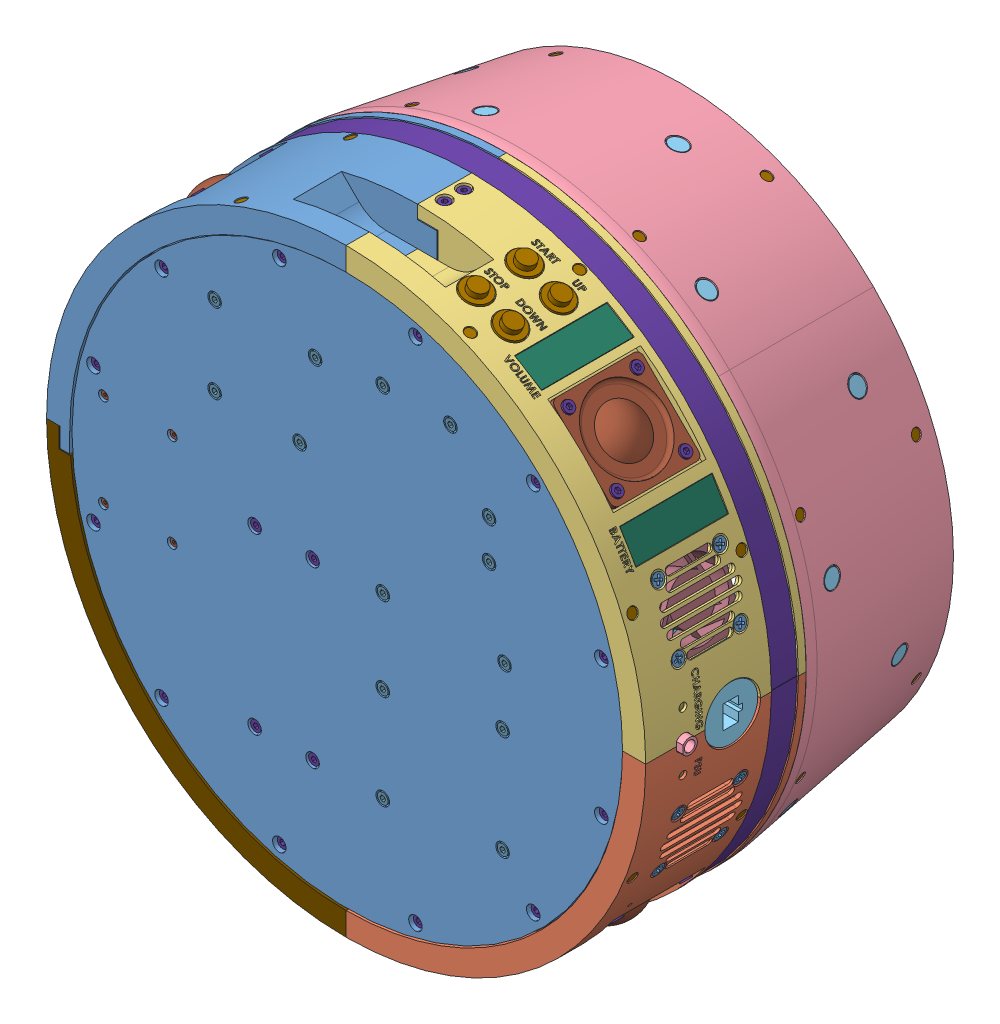
SolidWorks assembly base, configuration Défaut. Lengths in mm.
Overall size (438.41 438.41 173).
296 component instances, 45 part files, 31 mates.
Components (placement in the parent):
- base disk-1: base disk [Défaut] at (36.9194 20.0613 317) size (285 285 66.55)
  - base disk-1: base disk [Défaut] at (-39.9498 -9.3034 266.18) size (285 285 6.35)
  - Adafruit MAX9744-1: Adafruit MAX9744 [Défaut] at (-148.3839 -9.3034 256.18) x (0 1 0) z (0 0 -1) size (56.74 43.64 13.6)
  - Adafruit MAX9744-2: Adafruit MAX9744 [Défaut] at (-148.3839 -9.3034 239.58) x (0 1 0) z (0 0 -1) size (56.74 43.64 13.6)
  - Battery charger RRC-PMM240-1: Battery charger RRC-PMM240 [Défaut] at (-52.8471 67.1868 256.18) x (0 -1 0) z (0 0 -1) size (57 70 12)
  - battery holder-1: battery holder [Défaut] at (-92.9498 0.6966 266.18) x (0 -1 0) z (1 0 0) size (115 36.2 40)
  - Battery RRC2054-2-1: Battery RRC2054-2 [Défaut] at (-82.3791 -10.7125 233.18) x (0 1 0) z (0 0 1) size (151 78 23)
  - ground loop noise isolator-1: ground loop noise isolator [Défaut] at (-105.1098 -100.3034 233.18) x (0 -1 0) z (1 0 0) size (20 20 60)
  - ground loop noise isolator-2: ground loop noise isolator [Défaut] at (-45.1098 -80.3034 233.18) x (0 0 1) z (-1 0 0) size (20 20 60)
  - psu control-1: psu control [Défaut] at (-25.1498 95.1966 256.18) x (0 -1 0) z (0 0 -1) size (100 70 16.5)
  - buck boost-1: buck boost [Défaut] at (-25.6498 -27.3034 256.18) x (0 -1 0) z (0 0 -1) size (80 70 23.6)
  - buck boost-2: buck boost [Défaut] at (-25.6498 -27.3034 229.58) x (0 -1 0) z (0 0 -1) size (80 70 23.6)
  - 732-12936-ND-1: 732-12936-ND [Défaut] at (-166.1639 14.8266 254.58) x (-0.923728 -0.383049 0) z (0 0 -1) size (4.6 4.17 20)
  - 732-12936-ND-2: 732-12936-ND [Défaut] at (-166.1639 -33.4334 254.58) x (-0.923728 -0.383049 0) z (0 0 -1) size (4.6 4.17 20)
  - 732-12936-ND-3: 732-12936-ND [Défaut] at (-130.6039 -33.4334 254.58) x (-0.923728 -0.383049 0) z (0 0 -1) size (4.6 4.17 20)
  - 732-12936-ND-4: 732-12936-ND [Défaut] at (-130.6039 14.8266 254.58) x (-0.923728 -0.383049 0) z (0 0 -1) size (4.6 4.17 20)
  - 732-12918-ND-1: 732-12918-ND [Défaut] at (-166.1639 14.8266 266.18) x (-0.923728 -0.383049 0) z (0 0 -1) size (4.6 4.17 15)
  - 732-12918-ND-2: 732-12918-ND [Défaut] at (-130.6039 14.8266 266.18) x (-0.923728 -0.383049 0) z (0 0 -1) size (4.6 4.17 15)
  - 732-12918-ND-3: 732-12918-ND [Défaut] at (-130.6039 -33.4334 266.18) x (-0.923728 -0.383049 0) z (0 0 -1) size (4.6 4.17 15)
  - 732-12918-ND-4: 732-12918-ND [Défaut] at (-166.1639 -33.4334 266.18) x (-0.923728 -0.383049 0) z (0 0 -1) size (4.6 4.17 15)
  - M2x8mm socket-6: M2x8mm socket [Défaut] at (-166.1639 -33.4334 262.03) x (-1 0 0) z (0 0 1) size (3.8 3.8 9.6)
  - M2x8mm socket-5: M2x8mm socket [Défaut] at (-130.6039 -33.4334 262.03) x (-1 0 0) z (0 0 1) size (3.8 3.8 9.6)
  - M2x8mm socket-3: M2x8mm socket [Défaut] at (-166.1639 14.8266 262.03) size (3.8 3.8 9.6)
  - M2x8mm socket-4: M2x8mm socket [Défaut] at (-130.6039 14.8266 262.03) x (-1 0 0) z (0 0 1) size (3.8 3.8 9.6)
  - M2 nut-1: M2 nut [Défaut] at (-166.1639 14.8266 237.98) x (-0.923728 -0.383049 0) z (0 0 -1) size (4.62 4 1.6)
  - M2 nut-2: M2 nut [Défaut] at (-166.1639 -33.4334 237.98) x (-0.923728 -0.383049 0) z (0 0 -1) size (4.62 4 1.6)
  - M2 nut-3: M2 nut [Défaut] at (-130.6039 -33.4334 237.98) x (-0.923728 -0.383049 0) z (0 0 -1) size (4.62 4 1.6)
  - M2 nut-4: M2 nut [Défaut] at (-130.6039 14.8266 237.98) x (-0.923728 -0.383049 0) z (0 0 -1) size (4.62 4 1.6)
  - 36-24337-ND-1: 36-24337-ND [Défaut] at (-108.6498 86.6966 266.18) x (-0.923728 -0.383049 0) z (0 0 -1) size (5.77 5 18)
  - 36-24337-ND-2: 36-24337-ND [Défaut] at (-108.6498 45.6966 266.18) x (-0.923728 -0.383049 0) z (0 0 -1) size (5.77 5 18)
  - 36-24337-ND-3: 36-24337-ND [Défaut] at (-64.6498 44.6966 266.18) x (-0.923728 -0.383049 0) z (0 0 -1) size (5.77 5 18)
  - 36-24337-ND-4: 36-24337-ND [Défaut] at (-56.6498 86.6966 266.18) x (-0.923728 -0.383049 0) z (0 0 -1) size (5.77 5 18)
  - M3x5mm socket-1: M3x5mm socket [Défaut] at (-108.6498 86.6966 264.53) x (-1 0 0) z (0 0 1) size (5.5 5.5 8)
  - M3x5mm socket-2: M3x5mm socket [Défaut] at (-108.6498 45.6966 264.53) x (-1 0 0) z (0 0 1) size (5.5 5.5 8)
  - M3x5mm socket-3: M3x5mm socket [Défaut] at (-64.6498 44.6966 264.53) x (-1 0 0) z (0 0 1) size (5.5 5.5 8)
  - M3x5mm socket-4: M3x5mm socket [Défaut] at (-56.6498 86.6966 264.53) x (-1 0 0) z (0 0 1) size (5.5 5.5 8)
  - M3 nut-1: M3 nut [Défaut] at (-108.6498 86.6966 254.18) x (-0.923728 -0.383049 0) z (0 0 -1) size (6.35 5.5 2.4)
  - M3 nut-2: M3 nut [Défaut] at (-108.6498 45.6966 254.18) x (-0.923728 -0.383049 0) z (0 0 -1) size (6.35 5.5 2.4)
  - M3 nut-3: M3 nut [Défaut] at (-64.6498 44.6966 254.18) x (-0.923728 -0.383049 0) z (0 0 -1) size (6.35 5.5 2.4)
  - M3 nut-4: M3 nut [Défaut] at (-56.6498 86.6966 254.18) x (-0.923728 -0.383049 0) z (0 0 -1) size (6.35 5.5 2.4)
  - 36-24337-ND-5: 36-24337-ND [Défaut] at (-21.6498 91.6966 266.18) x (-0.923728 -0.383049 0) z (0 0 -1) size (5.77 5 18)
  - 36-24337-ND-6: 36-24337-ND [Défaut] at (-21.6498 -1.3034 266.18) x (1 0 0) z (0 0 -1) size (5.77 5 18)
  - 36-24337-ND-7: 36-24337-ND [Défaut] at (13.3502 91.6966 266.18) x (0.923728 0.383049 0) z (0 0 -1) size (5.77 5 18)
  - 36-24337-ND-8: 36-24337-ND [Défaut] at (41.3502 -1.3034 266.18) x (-1 0 0) z (0 0 -1) size (5.77 5 18)
  - M3 nut-5: M3 nut [Défaut] at (-21.6498 91.6966 256.98) x (-1 0 0) z (0 0 -1) size (6.35 5.5 2.4)
  - M3 nut-6: M3 nut [Défaut] at (13.3502 91.6966 252.18) x (-1 0 0) z (0 0 1) size (6.35 5.5 2.4)
  - M3 nut-7: M3 nut [Défaut] at (-21.6498 -1.3034 252.18) x (-1 0 0) z (0 0 1) size (6.35 5.5 2.4)
  - M3 nut-8: M3 nut [Défaut] at (41.3502 -1.3034 252.18) size (6.35 5.5 2.4)
  - 36-24337-ND-9: 36-24337-ND [Défaut] at (-21.6498 -44.3034 266.18) x (-0.923728 -0.383049 0) z (0 0 -1) size (5.77 5 18)
  - 36-24337-ND-10: 36-24337-ND [Défaut] at (-21.6498 -93.3034 266.18) x (-0.923728 -0.383049 0) z (0 0 -1) size (5.77 5 18)
  - 36-24337-ND-11: 36-24337-ND [Défaut] at (40.3502 -85.3034 266.18) x (-0.923728 -0.383049 0) z (0 0 -1) size (5.77 5 18)
  - 36-24337-ND-12: 36-24337-ND [Défaut] at (40.3502 -31.3034 266.18) x (-0.923728 -0.383049 0) z (0 0 -1) size (5.77 5 18)
  - 36-24342-ND-1: 36-24342-ND [Défaut] at (-21.6498 -44.3034 254.58) x (1 0 0) z (0 0 -1) size (5.77 5 33)
  - 36-24342-ND-2: 36-24342-ND [Défaut] at (-21.6498 -93.3034 254.58) x (1 0 0) z (0 0 -1) size (5.77 5 33)
  - 36-24342-ND-3: 36-24342-ND [Défaut] at (40.3502 -31.3034 254.58) x (1 0 0) z (0 0 -1) size (5.77 5 33)
  - 36-24342-ND-4: 36-24342-ND [Défaut] at (40.3502 -85.3034 254.58) x (1 0 0) z (0 0 -1) size (5.77 5 33)
  - M3 nut-9: M3 nut [Défaut] at (40.3502 -31.3034 227.98) x (-1 0 0) z (0 0 -1) size (6.35 5.5 2.4)
  - M3 nut-10: M3 nut [Défaut] at (-21.6498 -44.3034 227.98) x (-1 0 0) z (0 0 -1) size (6.35 5.5 2.4)
  - M3 nut-11: M3 nut [Défaut] at (-21.6498 -93.3034 225.58) size (6.35 5.5 2.4)
  - M3 nut-12: M3 nut [Défaut] at (40.3502 -85.3034 227.98) x (-1 0 0) z (0 0 -1) size (6.35 5.5 2.4)
  - 36-24337-ND-13: 36-24337-ND [Défaut] at (33.3502 60.1966 266.18) x (-0.923728 -0.383049 0) z (0 0 -1) size (5.77 5 18)
  - 36-24337-ND-14: 36-24337-ND [Défaut] at (33.3502 40.1966 266.18) x (-0.923728 -0.383049 0) z (0 0 -1) size (5.77 5 18)
  - M3 nut-13: M3 nut [Défaut] at (33.3502 60.1966 252.18) size (6.35 5.5 2.4)
  - M3 nut-14: M3 nut [Défaut] at (33.3502 40.1966 252.18) size (6.35 5.5 2.4)
  - M3x8mm plastic-1: M3x8mm plastic [Défaut] at (-57.9498 -4.3034 261.53) size (5.5 5.5 10.3)
  - M3x8mm plastic-2: M3x8mm plastic [Défaut] at (-57.9498 -94.3034 261.53) size (5.5 5.5 10.3)
  - M3x8mm plastic-3: M3x8mm plastic [Défaut] at (-87.9498 -94.3034 261.53) size (5.5 5.5 10.3)
  - M3x8mm plastic-4: M3x8mm plastic [Défaut] at (-87.9498 -4.3034 261.53) size (5.5 5.5 10.3)
  - M3x5mm socket-5: M3x5mm socket [Défaut] at (-21.6498 91.6966 264.53) size (5.5 5.5 8)
  - M3x5mm socket-6: M3x5mm socket [Défaut] at (13.3502 91.6966 264.53) size (5.5 5.5 8)
  - M3x5mm socket-7: M3x5mm socket [Défaut] at (33.3502 60.1966 264.53) size (5.5 5.5 8)
  - M3x5mm socket-8: M3x5mm socket [Défaut] at (33.3502 40.1966 264.53) size (5.5 5.5 8)
  - M3x5mm socket-9: M3x5mm socket [Défaut] at (-21.6498 -1.3034 264.53) size (5.5 5.5 8)
  - M3x5mm socket-10: M3x5mm socket [Défaut] at (-21.6498 -44.3034 264.53) size (5.5 5.5 8)
  - M3x5mm socket-11: M3x5mm socket [Défaut] at (-21.6498 -93.3034 264.53) size (5.5 5.5 8)
  - M3x5mm socket-12: M3x5mm socket [Défaut] at (40.3502 -85.3034 264.53) size (5.5 5.5 8)
  - M3x5mm socket-13: M3x5mm socket [Défaut] at (40.3502 -31.3034 264.53) size (5.5 5.5 8)
  - M3x5mm socket-14: M3x5mm socket [Défaut] at (41.3502 -1.3034 264.53) size (5.5 5.5 8)
- base audio-1: base audio [Défaut] at (-77.1238 -92.9542 353.528) x (0 1 0) z (0 0 1) size (420.86 420.86 86)
  - base audio front left-1: base audio front left [Défaut] at (103.7122 -74.0934 171.652) size (155 165 86)
  - base audio front right-1: base audio front right [Défaut] at (103.7122 -74.0934 171.652) x (0 -1 0) z (0 0 1) size (165 165 86)
  - base audio back left-1: base audio back left [Défaut] at (103.7122 -74.0934 171.652) x (0 1 0) z (0 0 1) size (155 156 86)
  - base audio back right-1: base audio back right [Défaut] at (103.7122 -74.0934 171.652) x (-1 0 0) z (0 0 1) size (156 155 86)
  - SC2073-ND-1: SC2073-ND [Défaut] at (103.7122 -222.6934 217.152) x (1 0 0) z (0 -1 0) size (11.94 11.94 36.36)
  - RJ45 connector-1: RJ45 connector [Défaut] at (103.7122 -228.0934 191.652) x (1 0 0) z (0 1 0) size (27.9 27.9 35.9)
  - Micro USB B (Adafruit 4217)-1: Micro USB B (Adafruit 4217) [Défaut] at (-6.0335 -126.2291 211.652) x (-0.429101 0.903257 0) z (0 0 1) size (28 33.5 28)
  - Micro USB B nut (Adafruit 4217)-1: Micro USB B nut (Adafruit 4217) [Défaut] at (-28.6149 -136.9566 211.652) x (0.18262 -0.384415 -0.904917) z (0.903257 0.429101 0) size (30.02 30.02 8)
  - switch-1: switch [Défaut] at (-36.2542 -140.9179 186.027) x (0.429101 -0.903257 0) z (0.903257 0.429101 0) size (20.75 14.7 24.67)
  - button-1: button [Défaut] at (254.7907 -122.0257 191.152) x (0.197389 0.622151 -0.757605) z (-0.953177 0.302412 0) size (14 14 27.8)
  - button-2: button [Défaut] at (247.8231 -140.0803 191.152) x (0.179537 0.392097 -0.902234) z (-0.909218 0.416321 0) size (14 14 27.8)
  - button-3: button [Défaut] at (254.7907 -122.0257 216.152) x (0.197389 0.622151 -0.757605) z (-0.953177 0.302412 0) size (14 14 27.8)
  - button-4: button [Défaut] at (247.8231 -140.0803 216.152) x (0.179537 0.392097 -0.902234) z (-0.909218 0.416321 0) size (14 14 27.8)
  - button nut-1: button nut [Défaut] at (247.1653 -119.6064 191.152) x (0.099317 0.313039 0.944533) z (-0.953177 0.302412 0) size (16 16 5)
  - button nut-2: button nut [Défaut] at (247.1653 -119.6064 216.152) x (0.099317 0.313039 0.944533) z (-0.953177 0.302412 0) size (16 16 5)
  - button nut-3: button nut [Défaut] at (240.5494 -136.7497 216.152) x (0.182325 0.398185 0.899003) z (-0.909218 0.416321 0) size (16 16 5)
  - button nut-4: button nut [Défaut] at (240.5494 -136.7497 191.152) x (0.179537 0.392097 -0.902234) z (-0.909218 0.416321 0) size (16 16 5) (hidden)
  - Dayton Audio DMA45-8-1: Dayton Audio DMA45-8 [Défaut] at (209.7782 -180.1594 199.652) x (0.707107 0.707107 0) z (0.707107 -0.707107 0) size (46 46 32.1)
  - Dayton Audio DMA45-8-2: Dayton Audio DMA45-8 [Défaut] at (209.7782 31.9727 199.652) x (-0.707107 0.707107 0) z (0.707107 0.707107 0) size (46 46 32.1)
  - Dayton Audio DMA45-8-3: Dayton Audio DMA45-8 [Défaut] at (-2.3539 31.9727 199.652) x (-0.707107 -0.707107 0) z (-0.707107 0.707107 0) size (46 46 32.1)
  - Dayton Audio DMA45-8-4: Dayton Audio DMA45-8 [Défaut] at (-2.3539 -180.1594 199.652) x (0.707107 -0.707107 0) z (-0.707107 -0.707107 0) size (46 46 32.1)
  - LED 5mm-1: LED 5mm [Défaut] at (88.5685 -227.8494 216.652) x (-0.876134 0.086292 -0.474281) z (0.098017 0.995185 0) size (5.5 5.5 18.7)
  - LED 5mm-2: LED 5mm [Défaut] at (118.8558 -227.8494 216.652) x (-0.780695 -0.076892 -0.620163) z (-0.098017 0.995185 0) size (5.5 5.5 18.7)
  - Noctua NF-A4X20-1: Noctua NF-A4X20 [Défaut] at (61.6633 -197.158 199.652) x (0.946287 -0.323328 0) z (-0.323328 -0.946287 0) size (39.9 39.9 19.95)
  - Noctua NF-A4X20-2: Noctua NF-A4X20 [Défaut] at (145.761 -197.158 199.652) x (0.946287 0.323328 0) z (0.323328 -0.946287 0) size (39.9 39.9 19.95)
  - LED level-1: LED level [Défaut] at (232.9084 -146.5387 181.6389) x (0.524024 0.851704 0) z (0.851704 -0.524024 0) size (12 34.5 2)
  - LED level-2: LED level [Défaut] at (185.0786 -197.8654 181.6389) x (0.857177 0.515023 0) z (0.515023 -0.857177 0) size (12 34.5 2)
  - LED level diffuser-1: LED level diffuser [Défaut] at (240.4553 -143.8142 199.2629) x (0.524024 0.851704 0) z (0.851704 -0.524024 0) size (16 47.5 1.59)
  - LED level diffuser-2: LED level diffuser [Défaut] at (193.0327 -198.9193 199.2629) x (0.857177 0.515023 0) z (0.515023 -0.857177 0) size (16 47.5 1.59)
  - LED strip-1: LED strip [Défaut] at (103.7122 -74.0934 159.902) x (0.707107 -0.707107 0) z (0 0 1) size (297.3 297.88 9.5)
  - LED strip diffuser (round)-1: LED strip diffuser (round) [Défaut] at (103.7122 -74.0934 157.902) x (0.000809 -1 0) z (0 0 1) size (309.17 309.17 13.5)
  - light sensor-1: light sensor [Défaut] at (228.5122 -87.4674 238.7403) x (0 0 -1) z (1 0 0) size (7.62 10.16 4.2)
  - light sensor-2: light sensor [Défaut] at (-21.0878 -87.4674 196.0637) x (0 0 1) z (-1 0 0) size (7.62 10.16 4.2)
  - light sensor-3: light sensor [Défaut] at (29.9331 -198.7828 198.0637) x (0 0 1) z (-0.537899 -0.843009 0) size (7.62 10.16 4.2)
  - light sensor-4: light sensor [Défaut] at (109.4763 70.6739 198.0637) x (0 0 1) z (0.073377 0.997304 0) size (7.62 10.16 4.2)
  - M3x8mm plastic-1: M3x8mm plastic [Défaut] at (98.7122 69.9066 183.652) x (1 0 0) z (0 1 0) size (5.5 5.5 10.3)
  - M3x8mm plastic-2: M3x8mm plastic [Défaut] at (98.7122 69.9066 213.652) x (1 0 0) z (0 1 0) size (5.5 5.5 10.3)
  - M3x8mm plastic-3: M3x8mm plastic [Défaut] at (-40.2878 -79.0934 180.652) x (0 0 1) z (-1 0 0) size (5.5 5.5 10.3)
  - M3x8mm plastic-4: M3x8mm plastic [Défaut] at (-40.2878 -79.0934 190.652) x (0 0 1) z (-1 0 0) size (5.5 5.5 10.3)
  - M3x8mm plastic-5: M3x8mm plastic [Défaut] at (247.7122 -79.0934 180.652) x (0 0 -1) z (1 0 0) size (5.5 5.5 10.3)
  - M3x8mm plastic-6: M3x8mm plastic [Défaut] at (247.7122 -79.0934 190.652) x (0 0 -1) z (1 0 0) size (5.5 5.5 10.3)
  - M3x8mm plastic-8: M3x8mm plastic [Défaut] at (192.6308 -188.1143 181.902) x (0.5 0.5 -0.707107) z (0.707107 -0.707107 0) size (5.5 5.5 10.3)
  - M3x8mm plastic-14: M3x8mm plastic [Défaut] at (-10.3088 -163.012 181.902) x (0.5 -0.5 -0.707107) z (-0.707107 -0.707107 0) size (5.5 5.5 10.3)
  - M3x8mm plastic-13: M3x8mm plastic [Défaut] at (14.7935 39.9276 181.902) x (-0.5 -0.5 -0.707107) z (-0.707107 0.707107 0) size (5.5 5.5 10.3)
  - M3x8mm plastic-12: M3x8mm plastic [Défaut] at (217.7331 14.8253 181.902) x (-0.5 0.5 -0.707107) z (0.707107 0.707107 0) size (5.5 5.5 10.3)
  - M3x8mm plastic-9: M3x8mm plastic [Défaut] at (217.7331 -163.012 217.402) x (0.5 0.5 -0.707107) z (0.707107 -0.707107 0) size (5.5 5.5 10.3)
  - M3x8mm plastic-17: M3x8mm plastic [Défaut] at (14.7935 -188.1143 217.402) x (0.5 -0.5 -0.707107) z (-0.707107 -0.707107 0) size (5.5 5.5 10.3)
  - M3x8mm plastic-16: M3x8mm plastic [Défaut] at (-10.3088 14.8253 217.402) x (-0.5 -0.5 -0.707107) z (-0.707107 0.707107 0) size (5.5 5.5 10.3)
  - M3x8mm plastic-15: M3x8mm plastic [Défaut] at (192.6308 39.9276 217.402) x (-0.5 0.5 -0.707107) z (0.707107 0.707107 0) size (5.5 5.5 10.3)
  - M3x8mm plastic-10: M3x8mm plastic [Défaut] at (192.6308 -188.1143 217.402) x (0.5 0.5 -0.707107) z (0.707107 -0.707107 0) size (5.5 5.5 10.3)
  - M3x8mm plastic-20: M3x8mm plastic [Défaut] at (-10.3088 -163.012 217.402) x (0.5 -0.5 -0.707107) z (-0.707107 -0.707107 0) size (5.5 5.5 10.3)
  - M3x8mm plastic-19: M3x8mm plastic [Défaut] at (14.7935 39.9276 217.402) x (-0.5 -0.5 -0.707107) z (-0.707107 0.707107 0) size (5.5 5.5 10.3)
  - M3x8mm plastic-18: M3x8mm plastic [Défaut] at (217.7331 14.8253 217.402) x (-0.5 0.5 -0.707107) z (0.707107 0.707107 0) size (5.5 5.5 10.3)
  - M3x8mm plastic-11: M3x8mm plastic [Défaut] at (217.7331 -163.012 181.902) x (0.5 0.5 -0.707107) z (0.707107 -0.707107 0) size (5.5 5.5 10.3)
  - M3x8mm plastic-23: M3x8mm plastic [Défaut] at (14.7935 -188.1143 181.902) x (0.5 -0.5 -0.707107) z (-0.707107 -0.707107 0) size (5.5 5.5 10.3)
  - M3x8mm plastic-22: M3x8mm plastic [Défaut] at (-10.3088 14.8253 181.902) x (-0.5 -0.5 -0.707107) z (-0.707107 0.707107 0) size (5.5 5.5 10.3)
  - M3x8mm plastic-21: M3x8mm plastic [Défaut] at (192.6308 39.9276 181.902) x (-0.5 0.5 -0.707107) z (0.707107 0.707107 0) size (5.5 5.5 10.3)
  - fan screw-1: fan screw [Défaut] at (165.5737 -205.6586 183.652) x (0.879667 0.300565 -0.368573) z (0.323328 -0.946287 0) size (6.3 6.3 9.5)
  - fan screw-2: fan screw [Défaut] at (165.5737 -205.6586 215.652) x (0.879667 0.300565 -0.368573) z (0.323328 -0.946287 0) size (6.3 6.3 9.5)
  - fan screw-3: fan screw [Défaut] at (135.2925 -216.0051 215.652) x (-0.927498 -0.316908 -0.198283) z (0.323328 -0.946287 0) size (6.3 6.3 9.5)
  - fan screw-4: fan screw [Défaut] at (135.2925 -216.0051 183.652) x (0.879667 0.300565 -0.368573) z (0.323328 -0.946287 0) size (6.3 6.3 9.5)
  - fan screw-5: fan screw [Défaut] at (72.1318 -216.0051 183.652) x (0.879667 -0.300565 0.368573) z (-0.323328 -0.946287 0) size (6.3 6.3 9.5)
  - fan screw-6: fan screw [Défaut] at (72.1318 -216.0051 215.652) x (0.879667 -0.300565 0.368573) z (-0.323328 -0.946287 0) size (6.3 6.3 9.5)
  - fan screw-7: fan screw [Défaut] at (41.8506 -205.6586 215.652) x (0.879667 -0.300565 0.368573) z (-0.323328 -0.946287 0) size (6.3 6.3 9.5)
  - fan screw-8: fan screw [Défaut] at (41.8506 -205.6586 183.652) x (0.879667 -0.300565 0.368573) z (-0.323328 -0.946287 0) size (6.3 6.3 9.5)
  - dewel pin 0.125in 0.5in-1: dewel pin 0.125in 0.5in [Défaut] at (111.2122 -212.8434 155.652) x (0 0 1) z (-1 0 0) size (3.17 3.17 12.7)
  - dewel pin 0.125in 0.5in-2: dewel pin 0.125in 0.5in [Défaut] at (111.2122 -223.0934 228.6844) x (0 0 1) z (-1 0 0) size (3.17 3.17 12.7)
  - M2x5mm plastic-1: M2x5mm plastic [Défaut] at (233.5122 -79.5934 217.402) x (0 0.924225 0.381849) z (-1 0 0) size (3.35 3.35 6.6)
  - M2x5mm plastic-2: M2x5mm plastic [Défaut] at (-26.0878 -79.5934 217.402) x (0 0.5 -0.866025) z (1 0 0) size (3.35 3.35 6.6)
  - M2x5mm plastic-3: M2x5mm plastic [Défaut] at (20.6058 -198.7624 219.402) x (-0.826053 0.527081 -0.199554) z (0.537899 0.843009 0) size (3.35 3.35 6.6)
  - M2x5mm plastic-4: M2x5mm plastic [Défaut] at (117.696 75.0827 219.402) x (0.994616 -0.073179 0.073377) z (-0.073377 -0.997304 0) size (3.35 3.35 6.6)
- base mic-1: base mic [Défaut] at (-78.91 184.7021 463.131) x (-0.707107 -0.707107 0) z (0.707107 -0.707107 0) size (310 92.85 310)
  - base mic-1: base mic [Défaut] at (69.3421 -41.049 176.652) size (155 90 160)
  - 8SoundsUSB Mic-1: 8SoundsUSB Mic [Défaut] at (30.5719 -34.8926 320.3049) x (0.980785 0 0.19509) z (-0.192688 0.156434 0.96871) size (25.4 23.4 21.48)
  - 8SoundsUSB Mic-2: 8SoundsUSB Mic [Défaut] at (-17.8103 6.4759 289.0854) x (0.83147 0 0.55557) z (-0.54873 0.156434 0.821233) size (25.4 23.4 21.48)
  - 8SoundsUSB Mic-3: 8SoundsUSB Mic [Défaut] at (-71.7864 6.4759 194.5283) x (0.19509 0 0.980785) z (-0.96871 0.156434 0.192688) size (25.4 23.4 21.48)
  - 8SoundsUSB Mic-4: 8SoundsUSB Mic [Défaut] at (-59.6505 -34.8926 250.8153) x (0.55557 0 0.83147) z (-0.821233 0.156434 0.54873) size (25.4 23.4 21.48)
  - 16SoundsUSB-1: 16SoundsUSB [Défaut] at (69.3421 -36.049 176.6521) x (1 0 0) z (0 -1 0) size (165.86 165.78 26.13)
  - M3x5mm plastic-1: M3x5mm plastic [Défaut] at (49.8528 -16.3964 325.89) x (-0.186611 0.963352 -0.192688) z (0.192688 -0.156434 -0.96871) size (5.5 5.5 7.3)
  - M3x5mm plastic-2: M3x5mm plastic [Défaut] at (30.2371 -16.3964 321.9882) x (-0.186611 0.963352 -0.192688) z (0.192688 -0.156434 -0.96871) size (5.5 5.5 7.3)
  - M3x5mm plastic-3: M3x5mm plastic [Défaut] at (49.3034 -34.1748 328.6517) x (-0.186611 0.963352 -0.192688) z (0.192688 -0.156434 -0.96871) size (5.5 5.5 7.3)
  - M3x5mm plastic-4: M3x5mm plastic [Défaut] at (29.6877 -34.1748 324.7499) x (-0.186611 0.963352 -0.192688) z (0.192688 -0.156434 -0.96871) size (5.5 5.5 7.3)
  - M3x5mm plastic-5: M3x5mm plastic [Défaut] at (-2.1344 24.9721 301.6238) x (-0.684341 0.480179 -0.54873) z (0.54873 -0.156434 -0.821233) size (5.5 5.5 7.3)
  - M3x5mm plastic-6: M3x5mm plastic [Défaut] at (-18.7638 24.9721 290.5124) x (-0.684341 0.480179 -0.54873) z (0.54873 -0.156434 -0.821233) size (5.5 5.5 7.3)
  - M3x5mm plastic-7: M3x5mm plastic [Défaut] at (-3.6988 7.1937 303.965) x (-0.684341 0.480179 -0.54873) z (0.54873 -0.156434 -0.821233) size (5.5 5.5 7.3)
  - M3x5mm plastic-8: M3x5mm plastic [Défaut] at (-20.3282 7.1937 292.8536) x (-0.684341 0.480179 -0.54873) z (0.54873 -0.156434 -0.821233) size (5.5 5.5 7.3)
  - M3x5mm plastic-9: M3x5mm plastic [Défaut] at (-49.9661 -16.3964 268.3981) x (-0.494502 0.284684 -0.821233) z (0.821233 -0.156434 -0.54873) size (5.5 5.5 7.3)
  - M3x5mm plastic-10: M3x5mm plastic [Défaut] at (-61.0775 -16.3964 251.7687) x (-0.494502 0.284684 -0.821233) z (0.821233 -0.156434 -0.54873) size (5.5 5.5 7.3)
  - M3x5mm plastic-11: M3x5mm plastic [Défaut] at (-63.4188 -34.1748 253.3331) x (-0.494502 0.284684 -0.821233) z (0.821233 -0.156434 -0.54873) size (5.5 5.5 7.3)
  - M3x5mm plastic-12: M3x5mm plastic [Défaut] at (-52.3074 -34.1748 269.9625) x (-0.494502 0.284684 -0.821233) z (0.821233 -0.156434 -0.54873) size (5.5 5.5 7.3)
  - M3x5mm plastic-13: M3x5mm plastic [Défaut] at (-72.3295 7.1937 215.0282) x (-0.225994 -0.876896 -0.424241) z (0.96871 -0.156434 -0.192688) size (5.5 5.5 7.3)
  - M3x5mm plastic-14: M3x5mm plastic [Défaut] at (-69.5678 24.9721 214.4788) x (-0.162376 0.187709 -0.96871) z (0.96871 -0.156434 -0.192688) size (5.5 5.5 7.3)
  - M3x5mm plastic-15: M3x5mm plastic [Défaut] at (-73.4696 24.9721 194.8631) x (-0.162376 0.187709 -0.96871) z (0.96871 -0.156434 -0.192688) size (5.5 5.5 7.3)
  - M3x5mm plastic-16: M3x5mm plastic [Défaut] at (-76.2313 7.1937 195.4125) x (-0.162376 0.187709 -0.96871) z (0.96871 -0.156434 -0.192688) size (5.5 5.5 7.3)
  - M3x8mm plastic-1: M3x8mm plastic [Défaut] at (15.9671 -42.4056 230.027) x (1 0 0) z (0 1 0) size (5.5 5.5 10.3)
  - M3x8mm plastic-2: M3x8mm plastic [Défaut] at (122.7171 -42.4056 230.027) x (1 0 0) z (0 1 0) size (5.5 5.5 10.3)
  - M3x8mm plastic-3: M3x8mm plastic [Défaut] at (15.9671 -42.4056 123.277) x (-0.837169 0 -0.546944) z (0 1 0) size (5.5 5.5 10.3)
  - M3x8mm plastic-4: M3x8mm plastic [Défaut] at (122.7171 -42.4056 123.277) x (-0.837169 0 -0.546944) z (0 1 0) size (5.5 5.5 10.3)
  - M3x5mm plastic-17: M3x5mm plastic [Défaut] at (-75.994 -16.3964 137.547) x (0.192688 0.963352 -0.186611) z (0.96871 -0.156434 0.192688) size (5.5 5.5 7.3)
  - M3x5mm plastic-18: M3x5mm plastic [Défaut] at (108.4472 -16.3964 31.3159) x (0.186611 0.963352 0.192688) z (-0.192688 -0.156434 0.96871) size (5.5 5.5 7.3)
  - M3x5mm plastic-19: M3x5mm plastic [Défaut] at (214.6783 -16.3964 215.7571) x (-0.192688 0.963352 0.186611) z (-0.96871 -0.156434 -0.192688) size (5.5 5.5 7.3)
  - M3x5mm plastic-20: M3x5mm plastic [Défaut] at (-82.6575 -34.1748 156.6133) x (0.192688 0.963352 -0.186611) z (0.96871 -0.156434 0.192688) size (5.5 5.5 7.3)
  - M3x5mm plastic-21: M3x5mm plastic [Défaut] at (89.3808 -34.1748 24.6524) x (0.186611 0.963352 0.192688) z (-0.192688 -0.156434 0.96871) size (5.5 5.5 7.3)
  - M3x5mm plastic-22: M3x5mm plastic [Défaut] at (221.3418 -34.1748 196.6907) x (-0.192688 0.963352 0.186611) z (-0.96871 -0.156434 -0.192688) size (5.5 5.5 7.3)
  - M3x5mm plastic-23: M3x5mm plastic [Défaut] at (-78.7557 -34.1748 136.9976) x (0.192688 0.963352 -0.186611) z (0.96871 -0.156434 0.192688) size (5.5 5.5 7.3)
  - M3x5mm plastic-24: M3x5mm plastic [Défaut] at (108.9965 -34.1748 28.5542) x (0.186611 0.963352 0.192688) z (-0.192688 -0.156434 0.96871) size (5.5 5.5 7.3)
  - M3x5mm plastic-25: M3x5mm plastic [Défaut] at (217.44 -34.1748 216.3064) x (-0.192688 0.963352 0.186611) z (-0.96871 -0.156434 -0.192688) size (5.5 5.5 7.3)
  - M3x5mm plastic-26: M3x5mm plastic [Défaut] at (-55.6296 24.9721 105.1755) x (0.54873 0.480179 -0.684341) z (0.821233 -0.156434 0.54873) size (5.5 5.5 7.3)
  - M3x5mm plastic-27: M3x5mm plastic [Défaut] at (140.8187 24.9721 51.6803) x (0.684341 0.480179 0.54873) z (-0.54873 -0.156434 0.821233) size (5.5 5.5 7.3)
  - M3x5mm plastic-28: M3x5mm plastic [Défaut] at (194.3139 24.9721 248.1286) x (-0.54873 0.480179 0.684341) z (-0.821233 -0.156434 -0.54873) size (5.5 5.5 7.3)
  - M3x5mm plastic-29: M3x5mm plastic [Défaut] at (-44.5182 24.9721 88.5461) x (0.54873 0.480179 -0.684341) z (0.821233 -0.156434 0.54873) size (5.5 5.5 7.3)
  - M3x5mm plastic-30: M3x5mm plastic [Défaut] at (157.4481 24.9721 62.7917) x (0.684341 0.480179 0.54873) z (-0.54873 -0.156434 0.821233) size (5.5 5.5 7.3)
  - M3x5mm plastic-31: M3x5mm plastic [Défaut] at (183.2025 24.9721 264.758) x (-0.54873 0.480179 0.684341) z (-0.821233 -0.156434 -0.54873) size (5.5 5.5 7.3)
  - M3x5mm plastic-32: M3x5mm plastic [Défaut] at (-57.9709 7.1937 103.6111) x (0.54873 0.480179 -0.684341) z (0.821233 -0.156434 0.54873) size (5.5 5.5 7.3)
  - M3x5mm plastic-33: M3x5mm plastic [Défaut] at (142.3831 7.1937 49.339) x (0.684341 0.480179 0.54873) z (-0.54873 -0.156434 0.821233) size (5.5 5.5 7.3)
  - M3x5mm plastic-34: M3x5mm plastic [Défaut] at (196.6551 7.1937 249.693) x (-0.54873 0.480179 0.684341) z (-0.821233 -0.156434 -0.54873) size (5.5 5.5 7.3)
  - M3x5mm plastic-35: M3x5mm plastic [Défaut] at (-46.8595 7.1937 86.9817) x (0.54873 0.480179 -0.684341) z (0.821233 -0.156434 0.54873) size (5.5 5.5 7.3)
  - M3x5mm plastic-36: M3x5mm plastic [Défaut] at (159.0125 7.1937 60.4504) x (0.684341 0.480179 0.54873) z (-0.54873 -0.156434 0.821233) size (5.5 5.5 7.3)
  - M3x5mm plastic-37: M3x5mm plastic [Défaut] at (185.5437 7.1937 266.3224) x (-0.54873 0.480179 0.684341) z (-0.821233 -0.156434 -0.54873) size (5.5 5.5 7.3)
  - M3x5mm plastic-38: M3x5mm plastic [Défaut] at (-22.404 -16.3964 57.3438) x (0.821233 0.284684 -0.494502) z (0.54873 -0.156434 0.821233) size (5.5 5.5 7.3)
  - M3x5mm plastic-39: M3x5mm plastic [Défaut] at (188.6504 -16.3964 84.9059) x (0.494502 0.284684 0.821233) z (-0.821233 -0.156434 0.54873) size (5.5 5.5 7.3)
  - M3x5mm plastic-40: M3x5mm plastic [Défaut] at (161.0882 -16.3964 295.9603) x (-0.821233 0.284684 0.494502) z (-0.54873 -0.156434 -0.821233) size (5.5 5.5 7.3)
  - M3x5mm plastic-41: M3x5mm plastic [Défaut] at (-5.7746 -16.3964 46.2324) x (0.821233 0.284684 -0.494502) z (0.54873 -0.156434 0.821233) size (5.5 5.5 7.3)
  - M3x5mm plastic-42: M3x5mm plastic [Défaut] at (199.7618 -16.3964 101.5353) x (0.494502 0.284684 0.821233) z (-0.821233 -0.156434 0.54873) size (5.5 5.5 7.3)
  - M3x5mm plastic-43: M3x5mm plastic [Défaut] at (144.4588 -16.3964 307.0717) x (-0.821233 0.284684 0.494502) z (-0.54873 -0.156434 -0.821233) size (5.5 5.5 7.3)
  - M3x5mm plastic-44: M3x5mm plastic [Défaut] at (-7.339 -34.1748 43.8911) x (0.821233 0.284684 -0.494502) z (0.54873 -0.156434 0.821233) size (5.5 5.5 7.3)
  - M3x5mm plastic-45: M3x5mm plastic [Défaut] at (202.103 -34.1748 99.9709) x (0.494502 0.284684 0.821233) z (-0.821233 -0.156434 0.54873) size (5.5 5.5 7.3)
  - M3x5mm plastic-46: M3x5mm plastic [Défaut] at (146.0232 -34.1748 309.4129) x (-0.821233 0.284684 0.494502) z (-0.54873 -0.156434 -0.821233) size (5.5 5.5 7.3)
  - M3x5mm plastic-47: M3x5mm plastic [Défaut] at (-23.9684 -34.1748 55.0025) x (0.821233 0.284684 -0.494502) z (0.54873 -0.156434 0.821233) size (5.5 5.5 7.3)
  - M3x5mm plastic-48: M3x5mm plastic [Défaut] at (190.9916 -34.1748 83.3415) x (0.494502 0.284684 0.821233) z (-0.821233 -0.156434 0.54873) size (5.5 5.5 7.3)
  - M3x5mm plastic-49: M3x5mm plastic [Défaut] at (162.6526 -34.1748 298.3015) x (-0.821233 0.284684 0.494502) z (-0.54873 -0.156434 -0.821233) size (5.5 5.5 7.3)
  - M3x5mm plastic-50: M3x5mm plastic [Défaut] at (30.966 7.1937 34.9804) x (0.424241 -0.876896 -0.225994) z (0.192688 -0.156434 0.96871) size (5.5 5.5 7.3)
  - M3x5mm plastic-51: M3x5mm plastic [Défaut] at (211.0138 7.1937 138.2759) x (0.225994 -0.876896 0.424241) z (-0.96871 -0.156434 0.192688) size (5.5 5.5 7.3)
  - M3x5mm plastic-52: M3x5mm plastic [Défaut] at (107.7183 7.1937 318.3237) x (-0.424241 -0.876896 0.225994) z (-0.192688 -0.156434 -0.96871) size (5.5 5.5 7.3)
  - M3x5mm plastic-53: M3x5mm plastic [Défaut] at (31.5153 24.9721 37.7421) x (0.96871 0.187709 -0.162376) z (0.192688 -0.156434 0.96871) size (5.5 5.5 7.3)
  - M3x5mm plastic-54: M3x5mm plastic [Défaut] at (208.252 24.9721 138.8252) x (0.162376 0.187709 0.96871) z (-0.96871 -0.156434 0.192688) size (5.5 5.5 7.3)
  - M3x5mm plastic-55: M3x5mm plastic [Défaut] at (107.1689 24.9721 315.5619) x (-0.96871 0.187709 0.162376) z (-0.192688 -0.156434 -0.96871) size (5.5 5.5 7.3)
  - M3x5mm plastic-56: M3x5mm plastic [Défaut] at (51.131 24.9721 33.8403) x (0.96871 0.187709 -0.162376) z (0.192688 -0.156434 0.96871) size (5.5 5.5 7.3)
  - M3x5mm plastic-57: M3x5mm plastic [Défaut] at (212.1539 24.9721 158.4409) x (0.162376 0.187709 0.96871) z (-0.96871 -0.156434 0.192688) size (5.5 5.5 7.3)
  - M3x5mm plastic-58: M3x5mm plastic [Défaut] at (87.5532 24.9721 319.4638) x (-0.96871 0.187709 0.162376) z (-0.192688 -0.156434 -0.96871) size (5.5 5.5 7.3)
  - M3x5mm plastic-59: M3x5mm plastic [Défaut] at (50.5817 7.1937 31.0786) x (0.96871 0.187709 -0.162376) z (0.192688 -0.156434 0.96871) size (5.5 5.5 7.3)
  - M3x5mm plastic-60: M3x5mm plastic [Défaut] at (214.9156 7.1937 157.8916) x (0.162376 0.187709 0.96871) z (-0.96871 -0.156434 0.192688) size (5.5 5.5 7.3)
  - M3x5mm plastic-61: M3x5mm plastic [Défaut] at (88.1026 7.1937 322.2255) x (-0.96871 0.187709 0.162376) z (-0.192688 -0.156434 -0.96871) size (5.5 5.5 7.3)
  - M3x5mm plastic-62: M3x5mm plastic [Défaut] at (-79.8958 -16.3964 157.1627) x (0.192688 0.963352 -0.186611) z (0.96871 -0.156434 0.192688) size (5.5 5.5 7.3)
  - M3x5mm plastic-63: M3x5mm plastic [Défaut] at (88.8315 -16.3964 27.4141) x (0.186611 0.963352 0.192688) z (-0.192688 -0.156434 0.96871) size (5.5 5.5 7.3)
  - M3x5mm plastic-64: M3x5mm plastic [Défaut] at (218.5801 -16.3964 196.1414) x (-0.192688 0.963352 0.186611) z (-0.96871 -0.156434 -0.192688) size (5.5 5.5 7.3)
  - 8SoundsUSB Mic-17: 8SoundsUSB Mic [Défaut] at (-4.8211 -34.8926 47.6594) x (-0.83147 0 0.55557) z (-0.54873 0.156434 -0.821233) size (25.4 23.4 21.48)
  - 8SoundsUSB Mic-18: 8SoundsUSB Mic [Défaut] at (198.3348 -34.8926 102.4888) x (-0.55557 0 -0.83147) z (0.821233 0.156434 -0.54873) size (25.4 23.4 21.48)
  - 8SoundsUSB Mic-19: 8SoundsUSB Mic [Défaut] at (143.5054 -34.8926 305.6447) x (0.83147 0 -0.55557) z (0.54873 0.156434 0.821233) size (25.4 23.4 21.48)
  - 8SoundsUSB Mic-20: 8SoundsUSB Mic [Défaut] at (51.4658 6.4759 35.5235) x (-0.980785 0 0.19509) z (-0.192688 0.156434 -0.96871) size (25.4 23.4 21.48)
  - 8SoundsUSB Mic-21: 8SoundsUSB Mic [Défaut] at (210.4706 6.4759 158.7758) x (-0.19509 0 -0.980785) z (0.96871 0.156434 -0.192688) size (25.4 23.4 21.48)
  - 8SoundsUSB Mic-22: 8SoundsUSB Mic [Défaut] at (87.2184 6.4759 317.7805) x (0.980785 0 -0.19509) z (0.192688 0.156434 0.96871) size (25.4 23.4 21.48)
  - 8SoundsUSB Mic-23: 8SoundsUSB Mic [Défaut] at (-43.0912 6.4759 89.4996) x (-0.55557 0 0.83147) z (-0.821233 0.156434 -0.54873) size (25.4 23.4 21.48)
  - 8SoundsUSB Mic-24: 8SoundsUSB Mic [Défaut] at (156.4946 6.4759 64.2187) x (-0.83147 0 -0.55557) z (0.54873 0.156434 -0.821233) size (25.4 23.4 21.48)
  - 8SoundsUSB Mic-25: 8SoundsUSB Mic [Défaut] at (181.7755 6.4759 263.8045) x (0.55557 0 -0.83147) z (0.821233 0.156434 0.54873) size (25.4 23.4 21.48)
  - 8SoundsUSB Mic-26: 8SoundsUSB Mic [Défaut] at (-74.3108 -34.8926 137.8818) x (-0.19509 0 0.980785) z (-0.96871 0.156434 -0.192688) size (25.4 23.4 21.48)
  - 8SoundsUSB Mic-27: 8SoundsUSB Mic [Défaut] at (108.1124 -34.8926 32.9991) x (-0.980785 0 -0.19509) z (0.192688 0.156434 -0.96871) size (25.4 23.4 21.48)
  - 8SoundsUSB Mic-28: 8SoundsUSB Mic [Défaut] at (212.995 -34.8926 215.4223) x (0.19509 0 -0.980785) z (0.96871 0.156434 0.192688) size (25.4 23.4 21.48)
  - base mic-5: base mic [Défaut] at (69.3421 -41.049 176.652) x (0 0 1) z (-1 0 0) size (155 90 160)
  - base mic-6: base mic [Défaut] at (69.3421 -41.049 176.652) x (-1 0 0) z (0 0 -1) size (155 90 160)
  - base mic-7: base mic [Défaut] at (69.3421 -41.049 176.652) x (0 0 -1) z (1 0 0) size (155 90 160)
- M3x8mm plastic-1: M3x8mm plastic [Défaut] at (93.1361 106.9245 577.53) size (5.5 5.5 10.3)
- M3x12mm plastic-1: M3x12mm plastic [Défaut] at (-55.8407 -116.7374 511.18) x (-0.923728 -0.383049 0) z (0 0 -1) size (5.5 5.5 14.3)
- M3x8mm plastic-13: M3x8mm plastic [Défaut] at (-3.0304 86.2416 505.5366) x (1 0 0) z (0 0 -1) size (5.5 5.5 10.3)
- M3x8mm plastic-14: M3x8mm plastic [Défaut] at (-78.5141 10.7579 505.5366) x (1 0 0) z (0 0 -1) size (5.5 5.5 10.3)
- M3x8mm plastic-15: M3x8mm plastic [Défaut] at (-3.0304 -64.7257 505.5366) x (1 0 0) z (0 0 -1) size (5.5 5.5 10.3)
- M3x8mm plastic-16: M3x8mm plastic [Défaut] at (72.4532 10.7579 505.5366) x (1 0 0) z (0 0 -1) size (5.5 5.5 10.3)
- magnet 5x1.6-1: magnet 5x1.6 [Défaut] at (-144.384 -47.7926 585.18) x (0.146447 -0.353553 0.92388) z (-0.92388 -0.382683 0) size (5 5 1.6)
- magnet 5x1.6-9: magnet 5x1.6 [Défaut] at (-56.9159 -119.3331 427.3698) x (-0.551357 0.357597 -0.753744) z (-0.377972 -0.912505 -0.156434) size (5 5 1.6)
- magnet 5x1.6-17: magnet 5x1.6 [Défaut] at (-61.1691 -129.6014 497.5426) x (-0.551357 0.357597 -0.753744) z (-0.377972 -0.912505 -0.156434) size (5 5 1.6)
- magnet 5x1.6-25: magnet 5x1.6 [Défaut] at (-144.384 -47.7926 528.68) x (0.146447 -0.353553 0.92388) z (-0.92388 -0.382683 0) size (5 5 1.6)
- M3x8mm plastic-2: M3x8mm plastic [Défaut] at (128.3355 45.9573 577.53) x (0.866025 -0.5 0) z (0 0 1) size (5.5 5.5 10.3)
- M3x8mm plastic-3: M3x8mm plastic [Défaut] at (128.3355 -24.4415 577.53) x (0.5 -0.866025 0) z (0 0 1) size (5.5 5.5 10.3)
- M3x8mm plastic-4: M3x8mm plastic [Défaut] at (93.1361 -85.4086 577.53) x (0 -1 0) z (0 0 1) size (5.5 5.5 10.3)
- M3x8mm plastic-5: M3x8mm plastic [Défaut] at (32.169 -120.608 577.53) x (-0.5 -0.866025 0) z (0 0 1) size (5.5 5.5 10.3)
- M3x8mm plastic-6: M3x8mm plastic [Défaut] at (-38.2298 -120.608 577.53) x (-0.866025 -0.5 0) z (0 0 1) size (5.5 5.5 10.3)
- M3x8mm plastic-7: M3x8mm plastic [Défaut] at (-99.1969 -85.4086 577.53) x (-1 0 0) z (0 0 1) size (5.5 5.5 10.3)
- M3x8mm plastic-8: M3x8mm plastic [Défaut] at (-134.3963 -24.4415 577.53) x (-0.866025 0.5 0) z (0 0 1) size (5.5 5.5 10.3)
- M3x8mm plastic-9: M3x8mm plastic [Défaut] at (-134.3963 45.9573 577.53) x (-0.5 0.866025 0) z (0 0 1) size (5.5 5.5 10.3)
- M3x8mm plastic-10: M3x8mm plastic [Défaut] at (-99.1969 106.9245 577.53) x (0 1 0) z (0 0 1) size (5.5 5.5 10.3)
- M3x8mm plastic-11: M3x8mm plastic [Défaut] at (-38.2298 142.1238 577.53) x (0.5 0.866025 0) z (0 0 1) size (5.5 5.5 10.3)
- M3x8mm plastic-12: M3x8mm plastic [Défaut] at (32.169 142.1238 577.53) x (0.866025 0.5 0) z (0 0 1) size (5.5 5.5 10.3)
- M3x12mm plastic-2: M3x12mm plastic [Défaut] at (49.7799 -116.7374 511.18) x (-0.382318 -0.924031 0) z (0 0 -1) size (5.5 5.5 14.3)
- M3x12mm plastic-3: M3x12mm plastic [Défaut] at (124.465 -42.0524 511.18) x (0.383049 -0.923728 0) z (0 0 -1) size (5.5 5.5 14.3)
- M3x12mm plastic-4: M3x12mm plastic [Défaut] at (124.465 63.5682 511.18) x (0.924031 -0.382318 0) z (0 0 -1) size (5.5 5.5 14.3)
- M3x12mm plastic-5: M3x12mm plastic [Défaut] at (49.7799 138.2533 511.18) x (0.923728 0.383049 0) z (0 0 -1) size (5.5 5.5 14.3)
- M3x12mm plastic-6: M3x12mm plastic [Défaut] at (-55.8407 138.2533 511.18) x (0.382318 0.924031 0) z (0 0 -1) size (5.5 5.5 14.3)
- M3x12mm plastic-7: M3x12mm plastic [Défaut] at (-130.5258 63.5682 511.18) x (-0.383049 0.923728 0) z (0 0 -1) size (5.5 5.5 14.3)
- M3x12mm plastic-8: M3x12mm plastic [Défaut] at (-130.5258 -42.0524 511.18) x (-0.924031 0.382318 0) z (0 0 -1) size (5.5 5.5 14.3)
- magnet 5x1.6-2: magnet 5x1.6 [Défaut] at (-144.384 69.3085 585.18) x (-0.146447 -0.353553 0.92388) z (-0.92388 0.382683 0) size (5 5 1.6)
- magnet 5x1.6-3: magnet 5x1.6 [Défaut] at (-61.581 152.1115 585.18) x (-0.353553 -0.146447 0.92388) z (-0.382683 0.92388 0) size (5 5 1.6)
- magnet 5x1.6-4: magnet 5x1.6 [Défaut] at (55.5202 152.1115 585.18) x (-0.353553 0.146447 0.92388) z (0.382683 0.92388 0) size (5 5 1.6)
- magnet 5x1.6-5: magnet 5x1.6 [Défaut] at (138.3232 69.3085 585.18) x (-0.146447 0.353553 0.92388) z (0.92388 0.382683 0) size (5 5 1.6)
- magnet 5x1.6-6: magnet 5x1.6 [Défaut] at (138.3232 -47.7926 585.18) x (0.146447 0.353553 0.92388) z (0.92388 -0.382683 0) size (5 5 1.6)
- magnet 5x1.6-7: magnet 5x1.6 [Défaut] at (55.5202 -130.5956 585.18) x (0.353553 0.146447 0.92388) z (0.382683 -0.92388 0) size (5 5 1.6)
- magnet 5x1.6-8: magnet 5x1.6 [Défaut] at (-61.581 -130.5956 585.18) x (0.353553 -0.146447 0.92388) z (-0.382683 -0.92388 0) size (5 5 1.6)
- magnet 5x1.6-10: magnet 5x1.6 [Défaut] at (-133.1214 -43.1275 427.3698) x (-0.137009 0.642728 -0.753744) z (-0.912505 -0.377972 -0.156434) size (5 5 1.6)
- magnet 5x1.6-11: magnet 5x1.6 [Défaut] at (-133.1214 64.6434 427.3698) x (0.357597 0.551357 -0.753744) z (-0.912505 0.377972 -0.156434) size (5 5 1.6)
- magnet 5x1.6-12: magnet 5x1.6 [Défaut] at (-56.9159 140.849 427.3698) x (0.642728 0.137009 -0.753744) z (-0.377972 0.912505 -0.156434) size (5 5 1.6)
- magnet 5x1.6-13: magnet 5x1.6 [Défaut] at (50.8551 140.849 427.3698) x (0.551357 -0.357597 -0.753744) z (0.377972 0.912505 -0.156434) size (5 5 1.6)
- magnet 5x1.6-14: magnet 5x1.6 [Défaut] at (127.0606 64.6434 427.3698) x (0.137009 -0.642728 -0.753744) z (0.912505 0.377972 -0.156434) size (5 5 1.6)
- magnet 5x1.6-15: magnet 5x1.6 [Défaut] at (127.0606 -43.1275 427.3698) x (-0.357597 -0.551357 -0.753744) z (0.912505 -0.377972 -0.156434) size (5 5 1.6)
- magnet 5x1.6-16: magnet 5x1.6 [Défaut] at (50.8551 -119.3331 427.3698) x (-0.642728 -0.137009 -0.753744) z (0.377972 -0.912505 -0.156434) size (5 5 1.6)
- magnet 5x1.6-18: magnet 5x1.6 [Défaut] at (-143.3897 -47.3808 497.5426) x (-0.137009 0.642728 -0.753744) z (-0.912505 -0.377972 -0.156434) size (5 5 1.6)
- magnet 5x1.6-19: magnet 5x1.6 [Défaut] at (-143.3897 68.8967 497.5426) x (0.357597 0.551357 -0.753744) z (-0.912505 0.377972 -0.156434) size (5 5 1.6)
- magnet 5x1.6-20: magnet 5x1.6 [Défaut] at (-61.1691 151.1172 497.5426) x (0.642728 0.137009 -0.753744) z (-0.377972 0.912505 -0.156434) size (5 5 1.6)
- magnet 5x1.6-21: magnet 5x1.6 [Défaut] at (55.1083 151.1172 497.5426) x (0.551357 -0.357597 -0.753744) z (0.377972 0.912505 -0.156434) size (5 5 1.6)
- magnet 5x1.6-22: magnet 5x1.6 [Défaut] at (137.3289 68.8967 497.5426) x (0.137009 -0.642728 -0.753744) z (0.912505 0.377972 -0.156434) size (5 5 1.6)
- magnet 5x1.6-23: magnet 5x1.6 [Défaut] at (137.3289 -47.3808 497.5426) x (-0.357597 -0.551357 -0.753744) z (0.912505 -0.377972 -0.156434) size (5 5 1.6)
- magnet 5x1.6-24: magnet 5x1.6 [Défaut] at (55.1083 -129.6014 497.5426) x (-0.642728 -0.137009 -0.753744) z (0.377972 -0.912505 -0.156434) size (5 5 1.6)
- magnet 5x1.6-26: magnet 5x1.6 [Défaut] at (-144.384 69.3085 528.68) x (-0.146447 -0.353553 0.92388) z (-0.92388 0.382683 0) size (5 5 1.6)
- magnet 5x1.6-27: magnet 5x1.6 [Défaut] at (-61.581 152.1115 528.68) x (-0.353553 -0.146447 0.92388) z (-0.382683 0.92388 0) size (5 5 1.6)
- magnet 5x1.6-28: magnet 5x1.6 [Défaut] at (55.5202 152.1115 528.68) x (-0.353553 0.146447 0.92388) z (0.382683 0.92388 0) size (5 5 1.6)
- magnet 5x1.6-29: magnet 5x1.6 [Défaut] at (138.3232 69.3085 528.68) x (-0.146447 0.353553 0.92388) z (0.92388 0.382683 0) size (5 5 1.6)
- magnet 5x1.6-30: magnet 5x1.6 [Défaut] at (138.3232 -47.7926 528.68) x (0.146447 0.353553 0.92388) z (0.92388 -0.382683 0) size (5 5 1.6)
- magnet 5x1.6-31: magnet 5x1.6 [Défaut] at (55.5202 -130.5956 528.68) x (0.353553 0.146447 0.92388) z (0.382683 -0.92388 0) size (5 5 1.6)
- magnet 5x1.6-32: magnet 5x1.6 [Défaut] at (-61.581 -130.5956 528.68) x (0.353553 -0.146447 0.92388) z (-0.382683 -0.92388 0) size (5 5 1.6)
Mates (geometry in assembly coordinates):
- Coïncidente1: coincident anti-aligned: plane of base disk-1/base disk-1 through (-3.0304 10.7579 583.18) normal (0 0 -1); plane of base audio-1/base audio front right-1 through (-3.0304 10.7579 583.18) normal (0 0 1)
- Coaxiale8: concentric aligned: cylinder of base audio-1/base audio back right-1 through (-3.0304 10.7579 590.18) axis (0 0 -1) radius 143; cylinder of base disk-1/base disk-1 through (-3.0304 10.7579 589.53) axis (0 0 -1) radius 142.5
- Parallèle4: parallel anti-aligned: plane of base disk-1/buck boost-1 through (81.2696 -67.2421 571.58) normal (1 0 0); plane of base audio-1/RJ45 connector-1 through (115.0696 10.7579 545.18) normal (-1 0 0)
- Coaxiale9: concentric aligned: cylinder of base disk-1/base disk-1 through (93.1361 106.9245 589.53) axis (0 0 -1) radius 1.75; cylinder of M3x8mm plastic-1 through (93.1361 106.9245 585.53) axis (0 0 -1) radius 1.5
- Coïncidente3: coincident aligned: plane of base disk-1/base disk-1 through (93.1361 106.9245 585.53) normal (0 0 1); circle of M3x8mm plastic-1
- Coïncidente71: coincident anti-aligned: plane of base audio-1/base audio front left-1 through (-3.0304 10.7579 504.18) normal (0 0 -1); plane of base mic-1/base mic-2 through (91.0148 104.8031 504.18) normal (0 0 1)
- Coïncidente72: coincident anti-aligned: plane of base audio-1/base audio front right-1 through (-3.0304 10.7579 504.18) normal (0 0 -1); plane of base mic-1/base mic-1 through (91.0148 -83.2873 504.18) normal (0 0 1)
- Coaxiale54: concentric anti-aligned: cylinder of base audio-1/base audio front right-1 through (-3.0304 10.7579 507.18) axis (0 0 -1) radius 144.5; cylinder of base mic-1/base mic-2 through (-3.0304 10.7579 504.18) axis (0 0 1) radius 145
- Coaxiale55: concentric aligned: cylinder of base audio-1/base audio front right-1 through (-130.5258 63.5682 590.181) axis (0 0 -1) radius 1.25; cylinder of base mic-1/base mic-3 through (-130.5258 63.5682 507.181) axis (0 0 -1) radius 1.75
- Coaxiale56: concentric anti-aligned: cylinder of base mic-1/base mic-4 through (-55.8407 -116.7374 507.181) axis (0 0 -1) radius 1.75; cylinder of M3x12mm plastic-1 through (-55.8407 -116.7374 499.18) axis (0 0 1) radius 1.5
- Coïncidente73: coincident aligned: plane of base mic-1/base mic-4 through (-97.0756 -83.2873 499.18) normal (0 0 -1); circle of M3x12mm plastic-1
- Coïncidente74: coincident: plane of base mic-1/base mic-2 through (89.2262 103.0145 427.18) normal (0 0 -1); plane of base gear-1/base gear 1-1 through (-111.0304 10.7579 427.18) normal (0 0 1)
- Coaxiale57: concentric aligned: cylinder of base mic-1/base mic-1 through (-3.0304 10.7579 504.18) axis (0 0 1) radius 138.4706; cylinder of base gear-1/base gear 4-1 through (-3.0304 10.7579 437.18) axis (0 0 1) radius 138
- Coaxiale58: concentric anti-aligned: cylinder of M3x8mm plastic-14 through (-78.5141 10.7579 497.5366) axis (0 0 1) radius 1.5; cylinder of base mic-1/base mic-3 through (-78.5141 10.7579 582.5913) axis (0 0 -1) radius 1.25
- Coïncidente75: coincident aligned: plane of base mic-1/16SoundsUSB-1 through (-60.3061 -46.5177 497.5366) normal (0 0 -1); circle of M3x8mm plastic-14
- Coaxiale59: concentric anti-aligned: cylinder of M3x8mm plastic-15 through (-3.0304 -64.7257 497.5366) axis (0 0 1) radius 1.5; cylinder of base mic-1/base mic-4 through (-3.0304 -64.7257 582.5913) axis (0 0 -1) radius 1.25
- Coïncidente77: coincident aligned: plane of base mic-1/16SoundsUSB-1 through (-60.3061 -46.5177 497.5366) normal (0 0 -1); circle of M3x8mm plastic-15
- Coaxiale60: concentric anti-aligned: cylinder of M3x8mm plastic-13 through (-3.0304 86.2416 497.5366) axis (0 0 1) radius 1.5; cylinder of base mic-1/base mic-2 through (-3.0304 86.2416 582.5913) axis (0 0 -1) radius 1.25
- Coïncidente78: coincident aligned: plane of base mic-1/16SoundsUSB-1 through (-60.3061 -46.5177 497.5366) normal (0 0 -1); circle of M3x8mm plastic-13
- Coaxiale61: concentric anti-aligned: cylinder of M3x8mm plastic-16 through (72.4532 10.7579 497.5366) axis (0 0 1) radius 1.5; cylinder of base mic-1/base mic-1 through (72.4532 10.7579 582.5913) axis (0 0 -1) radius 1.25
- Coïncidente79: coincident aligned: plane of base mic-1/16SoundsUSB-1 through (-60.3061 -46.5177 497.5366) normal (0 0 -1); circle of M3x8mm plastic-16
- Coïncidente80: coincident anti-aligned: plane of base audio-1/base audio front left-1 through (-144.384 -47.7926 585.18) normal (-0.92388 -0.382683 0); plane of magnet 5x1.6-1 through (-144.384 -47.7926 585.18) normal (0.92388 0.382683 0)
- Coaxiale62: concentric anti-aligned: cylinder of base audio-1/base audio front left-1 through (-144.384 -47.7926 585.18) axis (-0.92388 -0.382683 0) radius 2.75; cylinder of magnet 5x1.6-1 through (-145.8622 -48.4049 585.18) axis (0.92388 0.382683 0) radius 2.5
- Coïncidente81: coincident anti-aligned: plane of base mic-1/base mic-4 through (-56.9159 -119.3331 427.3698) normal (-0.377972 -0.912505 -0.156434); plane of magnet 5x1.6-9 through (-56.9159 -119.3331 427.3698) normal (0.377972 0.912505 0.156434)
- Coaxiale63: concentric anti-aligned: cylinder of base mic-1/base mic-4 through (-56.9159 -119.3331 427.3698) axis (-0.377972 -0.912505 -0.156434) radius 2.75; cylinder of magnet 5x1.6-9 through (-57.5206 -120.7931 427.1195) axis (0.377972 0.912505 0.156434) radius 2.5
- Coïncidente82: coincident anti-aligned: plane of base mic-1/base mic-4 through (-61.1691 -129.6014 497.5426) normal (-0.377972 -0.912505 -0.156434); plane of magnet 5x1.6-17 through (-61.1691 -129.6014 497.5426) normal (0.377972 0.912505 0.156434)
- Coaxiale64: concentric anti-aligned: cylinder of base mic-1/base mic-4 through (-61.1691 -129.6014 497.5426) axis (-0.377972 -0.912505 -0.156434) radius 2.75; cylinder of magnet 5x1.6-17 through (-61.7739 -131.0614 497.2923) axis (0.377972 0.912505 0.156434) radius 2.5
- Coïncidente83: coincident anti-aligned: plane of base audio-1/base audio front left-1 through (-144.384 -47.7926 528.68) normal (-0.92388 -0.382683 0); plane of magnet 5x1.6-25 through (-144.384 -47.7926 528.68) normal (0.92388 0.382683 0)
- Coaxiale65: concentric anti-aligned: cylinder of base audio-1/base audio front left-1 through (-144.384 -47.7926 528.68) axis (-0.92388 -0.382683 0) radius 2.75; cylinder of magnet 5x1.6-25 through (-145.8622 -48.4049 528.68) axis (0.92388 0.382683 0) radius 2.5
- Coaxiale70: concentric aligned: cylinder of base audio-1/base audio back left-1 through (-3.0304 10.7579 504.18) axis (0 0 1) radius 133; cylinder of base mic-1/base mic-1 through (-3.0304 10.7579 504.18) axis (0 0 1) radius 133
- Parallèle6: parallel: plane of base audio-1/RJ45 connector-1 through (115.0696 10.7579 545.18) normal (-1 0 0); line of base mic-1/base mic-1 through (129.758 18.2579 499.18) axis (0 -1 0)
